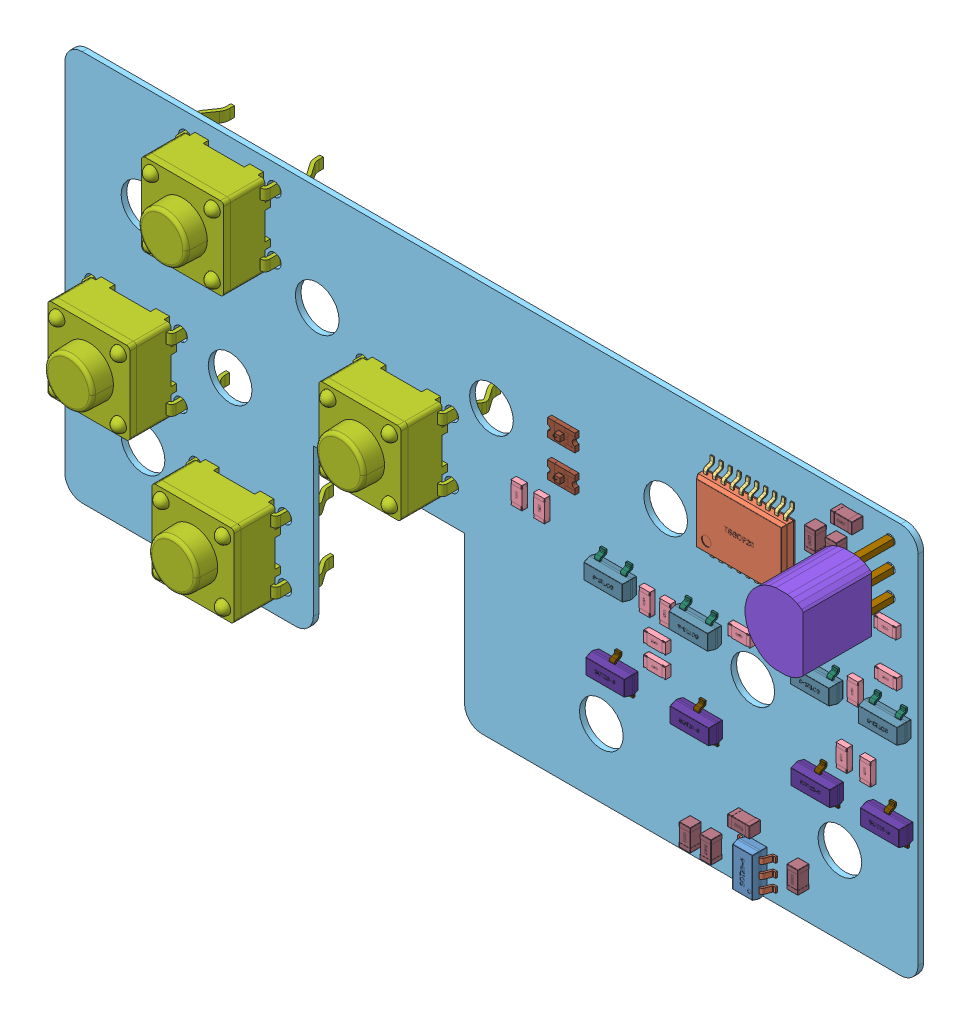
SolidWorks assembly DC_Card, configuration Default. Lengths in mm.
Overall size (62.36 28.58 11.46).
204 component instances, 23 part files, 0 mates.
Components (placement in the parent):
- DC_Card.step-1: DC_Card.step [默认] at origin size (62.36 28.58 11.46)
  - U2.step-1: U2.step [默认] at origin size (2.81 3 1.18)
    - 1167786160.step-1: 1167786160.step [默认] at (114.808 54.61 0) x (0 1 0) z (0 0 1) size (3 2.81 1.18)
      - SOT23-5.step-1: SOT23-5.step [默认] at origin size (3 1.6 1.1)
      - SOT23-5and6_____.step-1: SOT23-5and6_____.step [默认] at (-0.95 -0.8 0.675) x (-1 0 0) z (0 0 1) size (0.4 0.6 0.78)
      - SOT23-5and6_____.step-2: SOT23-5and6_____.step [默认] at (0 -0.8 0.675) x (-1 0 0) z (0 0 1) size (0.4 0.6 0.78)
      - SOT23-5and6_____.step-3: SOT23-5and6_____.step [默认] at (0.95 -0.8 0.675) x (-1 0 0) z (0 0 1) size (0.4 0.6 0.78)
      - SOT23-5and6_____.step-4: SOT23-5and6_____.step [默认] at (-0.95 0.8 0.675) size (0.4 0.6 0.78)
      - SOT23-5and6_____.step-5: SOT23-5and6_____.step [默认] at (0.95 0.8 0.675) size (0.4 0.6 0.78)
      - LOGO_0.15.step-1: LOGO_0.15.step [默认] at (0 -0.0167 0.0485) x (-1 0 0) z (0 0 -1) size (0.45 0.52 0)
  - R13.step-1: R13.step [默认] at origin size (1.6 0.8 0.4)
    - R_0603.step-1: R_0603.step [默认] at (124.46 74.549 0) x (-1 0 0) z (0 0 1) size (1.6 0.8 0.4)
      - R_0603-0.step-1: R_0603-0.step [默认] at origin size (1.6 0.8 0.4)
      - LOGO_.step-1: LOGO_.step [默认] at (0.0001 0.0322 -0.0016) x (-1 0 0) z (0 0 -1) size (0.48 0.55 0)
  - R12.step-1: R12.step [默认] at origin size (0.8 1.6 0.4)
    - R_0603.step-1: R_0603.step [默认] at (97.536 69.469 0) x (0 -1 0) z (0 0 1) size (1.6 0.8 0.4)
      - R_0603-0.step-1: R_0603-0.step [默认] at origin size (1.6 0.8 0.4)
      - LOGO_.step-1: LOGO_.step [默认] at (0.0001 0.0322 -0.0016) x (-1 0 0) z (0 0 -1) size (0.48 0.55 0)
  - R11.step-1: R11.step [默认] at origin size (0.8 1.6 0.4)
    - R_0603.step-1: R_0603.step [默认] at (99.187 69.469 0) x (0 -1 0) z (0 0 1) size (1.6 0.8 0.4)
      - R_0603-0.step-1: R_0603-0.step [默认] at origin size (1.6 0.8 0.4)
      - LOGO_.step-1: LOGO_.step [默认] at (0.0001 0.0322 -0.0016) x (-1 0 0) z (0 0 -1) size (0.48 0.55 0)
  - KEY4.step-1: KEY4.step [默认] at origin size (8.21 6 8.4)
    - TSW_DIP-6x6x5.step-1: TSW_DIP-6x6x5.step [默认] at (76.962 57.023 0.05) x (0 1 0) z (1 0 0) size (6 8.4 8.21)
      - LOGO_-1.step-1: LOGO_-1.step [默认] at (0.0186 0.396 1.2756) x (1 0 0) z (0 -1 0) size (1.2 1.38 0.01)
      - TSW_DIP-6x6x5-2.step-1: TSW_DIP-6x6x5-2.step [默认] at origin size (6 8.4 8.21)
  - KEY3.step-1: KEY3.step [默认] at origin size (8.21 6 8.4)
    - TSW_DIP-6x6x5.step-1: TSW_DIP-6x6x5.step [默认] at (69.342 64.77 0.05) x (0 1 0) z (1 0 0) size (6 8.4 8.21)
      - LOGO_-1.step-1: LOGO_-1.step [默认] at (0.0186 0.396 1.2756) x (1 0 0) z (0 -1 0) size (1.2 1.38 0.01)
      - TSW_DIP-6x6x5-2.step-1: TSW_DIP-6x6x5-2.step [默认] at origin size (6 8.4 8.21)
  - KEY2.step-1: KEY2.step [默认] at origin size (8.21 6 8.4)
    - TSW_DIP-6x6x5.step-1: TSW_DIP-6x6x5.step [默认] at (89.154 69.596 0.05) x (0 1 0) z (1 0 0) size (6 8.4 8.21)
      - LOGO_-1.step-1: LOGO_-1.step [默认] at (0.0186 0.396 1.2756) x (1 0 0) z (0 -1 0) size (1.2 1.38 0.01)
      - TSW_DIP-6x6x5-2.step-1: TSW_DIP-6x6x5-2.step [默认] at origin size (6 8.4 8.21)
  - KEY1.step-1: KEY1.step [默认] at origin size (8.21 6 8.4)
    - TSW_DIP-6x6x5.step-1: TSW_DIP-6x6x5.step [默认] at (76.2 77.343 0.05) x (0 1 0) z (1 0 0) size (6 8.4 8.21)
      - LOGO_-1.step-1: LOGO_-1.step [默认] at (0.0186 0.396 1.2756) x (1 0 0) z (0 -1 0) size (1.2 1.38 0.01)
      - TSW_DIP-6x6x5-2.step-1: TSW_DIP-6x6x5-2.step [默认] at origin size (6 8.4 8.21)
  - IR.step-1: IR.step [默认] at origin size (4.25 5.18 8.01)
    - 1126849328.step-1: 1126849328.step [默认] at (123.985 78.105 3) size (4.25 5.18 5.01)
      - Extruded.step-1: Extruded.step [默认] at origin size (4.25 5.18 5.01)
    - 1126849192.step-1: 1126849192.step [默认] at (124.46 76.2848 0) size (0.5 0.44 3)
      - Extruded-3.step-1: Extruded-3.step [默认] at origin size (0.5 0.44 3)
    - 1126849192.step-2: 1126849192.step [默认] at (124.46 78.105 0) size (0.5 0.44 3)
      - Extruded-3.step-1: Extruded-3.step [默认] at origin size (0.5 0.44 3)
    - 1126849192.step-3: 1126849192.step [默认] at (124.464 79.9084 0) size (0.5 0.44 3)
      - Extruded-3.step-1: Extruded-3.step [默认] at origin size (0.5 0.44 3)
  - DS1.step-1: DS1.step [默认] at origin size (2 1.25 0.67)
    - 1167786416.step-1: 1167786416.step [默认] at (100.711 74.803 0) x (-1 0 0) z (0 0 1) size (2 1.25 0.67)
      - LOGO_-4.step-1: LOGO_-4.step [默认] at (0 0.0303 -0.002) x (-1 0 0) z (0 0 -1) size (0.6 0.69 0)
      - LED_0805-R.step-1: LED_0805-R.step [默认] at origin size (2 1.25 0.67)
  - DS0.step-1: DS0.step [默认] at origin size (2 1.25 0.67)
    - 1167786416.step-1: 1167786416.step [默认] at (100.711 72.136 0) x (-1 0 0) z (0 0 1) size (2 1.25 0.67)
      - LOGO_-4.step-1: LOGO_-4.step [默认] at (0 0.0303 -0.002) x (-1 0 0) z (0 0 -1) size (0.6 0.69 0)
      - LED_0805-R.step-1: LED_0805-R.step [默认] at origin size (2 1.25 0.67)
  - C8.step-1: C8.step [默认] at origin size (0.82 1.6 0.82)
    - C_0603.step-1: C_0603.step [默认] at (111.76 54.356 0) x (0 -1 0) z (0 0 1) size (1.6 0.82 0.82)
      - LOGO_-5.step-1: LOGO_-5.step [默认] at (0 0.0171 -0.0006) x (-1 0 0) z (0 0 -1) size (0.51 0.59 0)
      - C_0603-6.step-1: C_0603-6.step [默认] at origin size (1.6 0.82 0.82)
  - C7.step-1: C7.step [默认] at origin size (0.82 1.6 0.82)
    - C_0603.step-1: C_0603.step [默认] at (110.236 54.356 0) x (0 -1 0) z (0 0 1) size (1.6 0.82 0.82)
      - LOGO_-5.step-1: LOGO_-5.step [默认] at (0 0.0171 -0.0006) x (-1 0 0) z (0 0 -1) size (0.51 0.59 0)
      - C_0603-6.step-1: C_0603-6.step [默认] at origin size (1.6 0.82 0.82)
  - C6.step-1: C6.step [默认] at origin size (1.6 0.82 0.82)
    - C_0603.step-1: C_0603.step [默认] at (114.173 57.023 0) x (-1 0 0) z (0 0 1) size (1.6 0.82 0.82)
      - LOGO_-5.step-1: LOGO_-5.step [默认] at (0 0.0171 -0.0006) x (-1 0 0) z (0 0 -1) size (0.51 0.59 0)
      - C_0603-6.step-1: C_0603-6.step [默认] at origin size (1.6 0.82 0.82)
  - C5.step-1: C5.step [默认] at origin size (0.82 1.6 0.82)
    - C_0603.step-1: C_0603.step [默认] at (118.11 55.626 0) x (0 1 0) z (0 0 1) size (1.6 0.82 0.82)
      - LOGO_-5.step-1: LOGO_-5.step [默认] at (0 0.0171 -0.0006) x (-1 0 0) z (0 0 -1) size (0.51 0.59 0)
      - C_0603-6.step-1: C_0603-6.step [默认] at origin size (1.6 0.82 0.82)
  - C3.step-1: C3.step [默认] at origin size (1.6 0.82 0.82)
    - C_0603.step-1: C_0603.step [默认] at (121.666 80.01 0) x (1 0 0) z (0 0 1) size (1.6 0.82 0.82)
      - LOGO_-5.step-1: LOGO_-5.step [默认] at (0 0.0171 -0.0006) x (-1 0 0) z (0 0 -1) size (0.51 0.59 0)
      - C_0603-6.step-1: C_0603-6.step [默认] at origin size (1.6 0.82 0.82)
  - C2.step-1: C2.step [默认] at origin size (0.82 1.6 0.82)
    - C_0603.step-1: C_0603.step [默认] at (120.904 77.724 0) x (0 1 0) z (0 0 1) size (1.6 0.82 0.82)
      - LOGO_-5.step-1: LOGO_-5.step [默认] at (0 0.0171 -0.0006) x (-1 0 0) z (0 0 -1) size (0.51 0.59 0)
      - C_0603-6.step-1: C_0603-6.step [默认] at origin size (1.6 0.82 0.82)
  - C1.step-1: C1.step [默认] at origin size (0.82 1.6 0.82)
    - C_0603.step-1: C_0603.step [默认] at (119.38 77.724 0) x (0 1 0) z (0 0 1) size (1.6 0.82 0.82)
      - LOGO_-5.step-1: LOGO_-5.step [默认] at (0 0.0171 -0.0006) x (-1 0 0) z (0 0 -1) size (0.51 0.59 0)
      - C_0603-6.step-1: C_0603-6.step [默认] at origin size (1.6 0.82 0.82)
  - Q1.step-1: Q1.step [默认] at origin size (3 2.4 1.05)
    - 1163770928.step-1: 1163770928.step [默认] at (119.6086 68.7488 0) x (-1 0 0) z (0 0 1) size (3 2.4 1.05)
      - SOT23-3.step-1: SOT23-3.step [默认] at origin size (3 1.3 1)
      - SOT23-3_____.step-1: SOT23-3_____.step [默认] at (0 0.5461 0.475) size (0.4 0.65 0.55)
      - SOT23-3_____.step-2: SOT23-3_____.step [默认] at (-0.95 -0.5461 0.475) x (-1 0 0) z (0 0 1) size (0.4 0.65 0.55)
      - SOT23-3_____.step-3: SOT23-3_____.step [默认] at (0.95 -0.5461 0.475) x (-1 0 0) z (0 0 1) size (0.4 0.65 0.55)
      - LOGO_0.15-7.step-1: LOGO_0.15-7.step [默认] at (0 -0.0163 0.0485) x (-1 0 0) z (0 0 -1) size (0.45 0.52 0)
  - Q2.step-1: Q2.step [默认] at origin size (3 2.4 1.05)
    - 1163770928.step-1: 1163770928.step [默认] at (104.521 67.7836 0) x (-1 0 0) z (0 0 1) size (3 2.4 1.05)
      - SOT23-3.step-1: SOT23-3.step [默认] at origin size (3 1.3 1)
      - SOT23-3_____.step-1: SOT23-3_____.step [默认] at (0 0.5461 0.475) size (0.4 0.65 0.55)
      - SOT23-3_____.step-2: SOT23-3_____.step [默认] at (-0.95 -0.5461 0.475) x (-1 0 0) z (0 0 1) size (0.4 0.65 0.55)
      - SOT23-3_____.step-3: SOT23-3_____.step [默认] at (0.95 -0.5461 0.475) x (-1 0 0) z (0 0 1) size (0.4 0.65 0.55)
      - LOGO_0.15-7.step-1: LOGO_0.15-7.step [默认] at (0 -0.0163 0.0485) x (-1 0 0) z (0 0 -1) size (0.45 0.52 0)
  - Q3.step-1: Q3.step [默认] at origin size (3 2.4 1.05)
    - 1163770928.step-1: 1163770928.step [默认] at (124.587 68.7488 0) x (-1 0 0) z (0 0 1) size (3 2.4 1.05)
      - SOT23-3.step-1: SOT23-3.step [默认] at origin size (3 1.3 1)
      - SOT23-3_____.step-1: SOT23-3_____.step [默认] at (0 0.5461 0.475) size (0.4 0.65 0.55)
      - SOT23-3_____.step-2: SOT23-3_____.step [默认] at (-0.95 -0.5461 0.475) x (-1 0 0) z (0 0 1) size (0.4 0.65 0.55)
      - SOT23-3_____.step-3: SOT23-3_____.step [默认] at (0.95 -0.5461 0.475) x (-1 0 0) z (0 0 1) size (0.4 0.65 0.55)
      - LOGO_0.15-7.step-1: LOGO_0.15-7.step [默认] at (0 -0.0163 0.0485) x (-1 0 0) z (0 0 -1) size (0.45 0.52 0)
  - Q4.step-1: Q4.step [默认] at origin size (3 2.4 1.05)
    - 1163770928.step-1: 1163770928.step [默认] at (110.744 67.7836 0) x (-1 0 0) z (0 0 1) size (3 2.4 1.05)
      - SOT23-3.step-1: SOT23-3.step [默认] at origin size (3 1.3 1)
      - SOT23-3_____.step-1: SOT23-3_____.step [默认] at (0 0.5461 0.475) size (0.4 0.65 0.55)
      - SOT23-3_____.step-2: SOT23-3_____.step [默认] at (-0.95 -0.5461 0.475) x (-1 0 0) z (0 0 1) size (0.4 0.65 0.55)
      - SOT23-3_____.step-3: SOT23-3_____.step [默认] at (0.95 -0.5461 0.475) x (-1 0 0) z (0 0 1) size (0.4 0.65 0.55)
      - LOGO_0.15-7.step-1: LOGO_0.15-7.step [默认] at (0 -0.0163 0.0485) x (-1 0 0) z (0 0 -1) size (0.45 0.52 0)
  - Q5.step-1: Q5.step [默认] at origin size (3 2.4 1.05)
    - 1163770800.step-1: 1163770800.step [默认] at (119.6594 62.3406 0) x (1 0 0) z (0 0 1) size (3 2.4 1.05)
      - SOT23-3-8.step-1: SOT23-3-8.step [默认] at origin size (3 1.3 1)
      - SOT23-3_____-9.step-1: SOT23-3_____-9.step [默认] at (0 0.5461 0.475) size (0.4 0.65 0.55)
      - SOT23-3_____-9.step-2: SOT23-3_____-9.step [默认] at (-0.95 -0.5461 0.475) x (-1 0 0) z (0 0 1) size (0.4 0.65 0.55)
      - SOT23-3_____-9.step-3: SOT23-3_____-9.step [默认] at (0.95 -0.5461 0.475) x (-1 0 0) z (0 0 1) size (0.4 0.65 0.55)
      - LOGO_0.15-10.step-1: LOGO_0.15-10.step [默认] at (0 -0.0163 0.0485) x (-1 0 0) z (0 0 -1) size (0.45 0.52 0)
  - Q6.step-1: Q6.step [默认] at origin size (3 2.4 1.05)
    - 1163770800.step-1: 1163770800.step [默认] at (104.6615 61.8326 0) x (1 0 0) z (0 0 1) size (3 2.4 1.05)
      - SOT23-3-8.step-1: SOT23-3-8.step [默认] at origin size (3 1.3 1)
      - SOT23-3_____-9.step-1: SOT23-3_____-9.step [默认] at (0 0.5461 0.475) size (0.4 0.65 0.55)
      - SOT23-3_____-9.step-2: SOT23-3_____-9.step [默认] at (-0.95 -0.5461 0.475) x (-1 0 0) z (0 0 1) size (0.4 0.65 0.55)
      - SOT23-3_____-9.step-3: SOT23-3_____-9.step [默认] at (0.95 -0.5461 0.475) x (-1 0 0) z (0 0 1) size (0.4 0.65 0.55)
      - LOGO_0.15-10.step-1: LOGO_0.15-10.step [默认] at (0 -0.0163 0.0485) x (-1 0 0) z (0 0 -1) size (0.45 0.52 0)
  - Q7.step-1: Q7.step [默认] at origin size (3 2.4 1.05)
    - 1163770800.step-1: 1163770800.step [默认] at (124.7275 62.3406 0) x (1 0 0) z (0 0 1) size (3 2.4 1.05)
      - SOT23-3-8.step-1: SOT23-3-8.step [默认] at origin size (3 1.3 1)
      - SOT23-3_____-9.step-1: SOT23-3_____-9.step [默认] at (0 0.5461 0.475) size (0.4 0.65 0.55)
      - SOT23-3_____-9.step-2: SOT23-3_____-9.step [默认] at (-0.95 -0.5461 0.475) x (-1 0 0) z (0 0 1) size (0.4 0.65 0.55)
      - SOT23-3_____-9.step-3: SOT23-3_____-9.step [默认] at (0.95 -0.5461 0.475) x (-1 0 0) z (0 0 1) size (0.4 0.65 0.55)
      - LOGO_0.15-10.step-1: LOGO_0.15-10.step [默认] at (0 -0.0163 0.0485) x (-1 0 0) z (0 0 -1) size (0.45 0.52 0)
  - Q8.step-1: Q8.step [默认] at origin size (3 2.4 1.05)
    - 1163770800.step-1: 1163770800.step [默认] at (110.8202 61.8326 0) x (1 0 0) z (0 0 1) size (3 2.4 1.05)
      - SOT23-3-8.step-1: SOT23-3-8.step [默认] at origin size (3 1.3 1)
      - SOT23-3_____-9.step-1: SOT23-3_____-9.step [默认] at (0 0.5461 0.475) size (0.4 0.65 0.55)
      - SOT23-3_____-9.step-2: SOT23-3_____-9.step [默认] at (-0.95 -0.5461 0.475) x (-1 0 0) z (0 0 1) size (0.4 0.65 0.55)
      - SOT23-3_____-9.step-3: SOT23-3_____-9.step [默认] at (0.95 -0.5461 0.475) x (-1 0 0) z (0 0 1) size (0.4 0.65 0.55)
      - LOGO_0.15-10.step-1: LOGO_0.15-10.step [默认] at (0 -0.0163 0.0485) x (-1 0 0) z (0 0 -1) size (0.45 0.52 0)
  - R1.step-1: R1.step [默认] at origin size (0.8 1.6 0.4)
    - R_0603.step-1: R_0603.step [默认] at (121.285 64.7192 0) x (0 1 0) z (0 0 1) size (1.6 0.8 0.4)
      - R_0603-0.step-1: R_0603-0.step [默认] at origin size (1.6 0.8 0.4)
      - LOGO_.step-1: LOGO_.step [默认] at (0.0001 0.0322 -0.0016) x (-1 0 0) z (0 0 -1) size (0.48 0.55 0)
  - R2.step-1: R2.step [默认] at origin size (0.8 1.6 0.4)
    - R_0603.step-1: R_0603.step [默认] at (123.0122 64.7192 0) x (0 1 0) z (0 0 1) size (1.6 0.8 0.4)
      - R_0603-0.step-1: R_0603-0.step [默认] at origin size (1.6 0.8 0.4)
      - LOGO_.step-1: LOGO_.step [默认] at (0.0001 0.0322 -0.0016) x (-1 0 0) z (0 0 -1) size (0.48 0.55 0)
  - R3.step-1: R3.step [默认] at origin size (0.8 1.6 0.4)
    - R_0603.step-1: R_0603.step [默认] at (122.0978 69.3166 0) x (0 1 0) z (0 0 1) size (1.6 0.8 0.4)
      - R_0603-0.step-1: R_0603-0.step [默认] at origin size (1.6 0.8 0.4)
      - LOGO_.step-1: LOGO_.step [默认] at (0.0001 0.0322 -0.0016) x (-1 0 0) z (0 0 -1) size (0.48 0.55 0)
  - R4.step-1: R4.step [默认] at origin size (1.6 0.8 0.4)
    - R_0603.step-1: R_0603.step [默认] at (124.5108 71.3486 0) x (1 0 0) z (0 0 1) size (1.6 0.8 0.4)
      - R_0603-0.step-1: R_0603-0.step [默认] at origin size (1.6 0.8 0.4)
      - LOGO_.step-1: LOGO_.step [默认] at (0.0001 0.0322 -0.0016) x (-1 0 0) z (0 0 -1) size (0.48 0.55 0)
  - R5.step-1: R5.step [默认] at origin size (1.6 0.8 0.4)
    - R_0603.step-1: R_0603.step [默认] at (107.6198 65.1764 0) x (1 0 0) z (0 0 1) size (1.6 0.8 0.4)
      - R_0603-0.step-1: R_0603-0.step [默认] at origin size (1.6 0.8 0.4)
      - LOGO_.step-1: LOGO_.step [默认] at (0.0001 0.0322 -0.0016) x (-1 0 0) z (0 0 -1) size (0.48 0.55 0)
  - R6.step-1: R6.step [默认] at origin size (1.6 0.8 0.4)
    - R_0603.step-1: R_0603.step [默认] at (107.6198 63.627 0) x (-1 0 0) z (0 0 1) size (1.6 0.8 0.4)
      - R_0603-0.step-1: R_0603-0.step [默认] at origin size (1.6 0.8 0.4)
      - LOGO_.step-1: LOGO_.step [默认] at (0.0001 0.0322 -0.0016) x (-1 0 0) z (0 0 -1) size (0.48 0.55 0)
  - R7.step-1: R7.step [默认] at origin size (0.8 1.6 0.4)
    - R_0603.step-1: R_0603.step [默认] at (106.8832 67.3862 0) x (0 1 0) z (0 0 1) size (1.6 0.8 0.4)
      - R_0603-0.step-1: R_0603-0.step [默认] at origin size (1.6 0.8 0.4)
      - LOGO_.step-1: LOGO_.step [默认] at (0.0001 0.0322 -0.0016) x (-1 0 0) z (0 0 -1) size (0.48 0.55 0)
  - R8.step-1: R8.step [默认] at origin size (0.8 1.6 0.4)
    - R_0603.step-1: R_0603.step [默认] at (108.3818 67.3862 0) x (0 1 0) z (0 0 1) size (1.6 0.8 0.4)
      - R_0603-0.step-1: R_0603-0.step [默认] at origin size (1.6 0.8 0.4)
      - LOGO_.step-1: LOGO_.step [默认] at (0.0001 0.0322 -0.0016) x (-1 0 0) z (0 0 -1) size (0.48 0.55 0)
  - R33.step-1: R33.step [默认] at origin size (1.6 0.8 0.4)
    - R_0603.step-1: R_0603.step [默认] at (113.792 68.707 0) x (1 0 0) z (0 0 1) size (1.6 0.8 0.4)
      - R_0603-0.step-1: R_0603-0.step [默认] at origin size (1.6 0.8 0.4)
      - LOGO_.step-1: LOGO_.step [默认] at (0.0001 0.0322 -0.0016) x (-1 0 0) z (0 0 -1) size (0.48 0.55 0)
  - R34.step-1: R34.step [默认] at origin size (1.6 0.8 0.4)
    - R_0603.step-1: R_0603.step [默认] at (116.5098 68.707 0) x (1 0 0) z (0 0 1) size (1.6 0.8 0.4)
      - R_0603-0.step-1: R_0603-0.step [默认] at origin size (1.6 0.8 0.4)
      - LOGO_.step-1: LOGO_.step [默认] at (0.0001 0.0322 -0.0016) x (-1 0 0) z (0 0 -1) size (0.48 0.55 0)
  - U1.step-1: U1.step [默认] at origin size (6.5 6.4 1.05)
    - TSSOP20.step-1: TSSOP20.step [默认] at (114.427 75.565 0) x (0 1 0) z (0 0 1) size (6.4 6.5 1.05)
      - TSSOP20_____.step-1: TSSOP20_____.step [默认] at origin size (4.6 6.5 1)
      - _____0.9.step-1: _____0.9.step [默认] at (2.3 -2.925 0.53) x (0 1 0) z (0 0 1) size (0.25 0.9 0.6)
      - _____0.9.step-2: _____0.9.step [默认] at (2.3 -2.275 0.53) x (0 1 0) z (0 0 1) size (0.25 0.9 0.6)
      - _____0.9.step-3: _____0.9.step [默认] at (2.3 -1.625 0.53) x (0 1 0) z (0 0 1) size (0.25 0.9 0.6)
      - _____0.9.step-4: _____0.9.step [默认] at (2.3 -0.975 0.53) x (0 1 0) z (0 0 1) size (0.25 0.9 0.6)
      - _____0.9.step-5: _____0.9.step [默认] at (2.3 -0.325 0.53) x (0 1 0) z (0 0 1) size (0.25 0.9 0.6)
      - _____0.9.step-6: _____0.9.step [默认] at (2.3 0.325 0.53) x (0 1 0) z (0 0 1) size (0.25 0.9 0.6)
      - _____0.9.step-7: _____0.9.step [默认] at (2.3 0.975 0.53) x (0 1 0) z (0 0 1) size (0.25 0.9 0.6)
      - _____0.9.step-8: _____0.9.step [默认] at (2.3 1.625 0.53) x (0 1 0) z (0 0 1) size (0.25 0.9 0.6)
      - _____0.9.step-9: _____0.9.step [默认] at (2.3 2.275 0.53) x (0 1 0) z (0 0 1) size (0.25 0.9 0.6)
      - _____0.9.step-10: _____0.9.step [默认] at (2.3 2.925 0.53) x (0 1 0) z (0 0 1) size (0.25 0.9 0.6)
      - _____0.9.step-11: _____0.9.step [默认] at (-2.3 -2.925 0.53) x (0 -1 0) z (0 0 1) size (0.25 0.9 0.6)
      - _____0.9.step-12: _____0.9.step [默认] at (-2.3 -2.275 0.53) x (0 -1 0) z (0 0 1) size (0.25 0.9 0.6)
      - _____0.9.step-13: _____0.9.step [默认] at (-2.3 -1.625 0.53) x (0 -1 0) z (0 0 1) size (0.25 0.9 0.6)
      - _____0.9.step-14: _____0.9.step [默认] at (-2.3 -0.975 0.53) x (0 -1 0) z (0 0 1) size (0.25 0.9 0.6)
      - _____0.9.step-15: _____0.9.step [默认] at (-2.3 -0.325 0.53) x (0 -1 0) z (0 0 1) size (0.25 0.9 0.6)
      - _____0.9.step-16: _____0.9.step [默认] at (-2.3 0.325 0.53) x (0 -1 0) z (0 0 1) size (0.25 0.9 0.6)
      - _____0.9.step-17: _____0.9.step [默认] at (-2.3 0.975 0.53) x (0 -1 0) z (0 0 1) size (0.25 0.9 0.6)
      - _____0.9.step-18: _____0.9.step [默认] at (-2.3 1.625 0.53) x (0 -1 0) z (0 0 1) size (0.25 0.9 0.6)
      - _____0.9.step-19: _____0.9.step [默认] at (-2.3 2.275 0.53) x (0 -1 0) z (0 0 1) size (0.25 0.9 0.6)
      - _____0.9.step-20: _____0.9.step [默认] at (-2.3 2.925 0.53) x (0 -1 0) z (0 0 1) size (0.25 0.9 0.6)
      - LOGO_0.25.step-1: LOGO_0.25.step [默认] at (-0.0065 0.1035 0.025) size (0.75 0.87 0.01)
  - Board.step-1: Board.step [默认] at (0 0 -0.4115) size (62.36 28.58 0.41)
